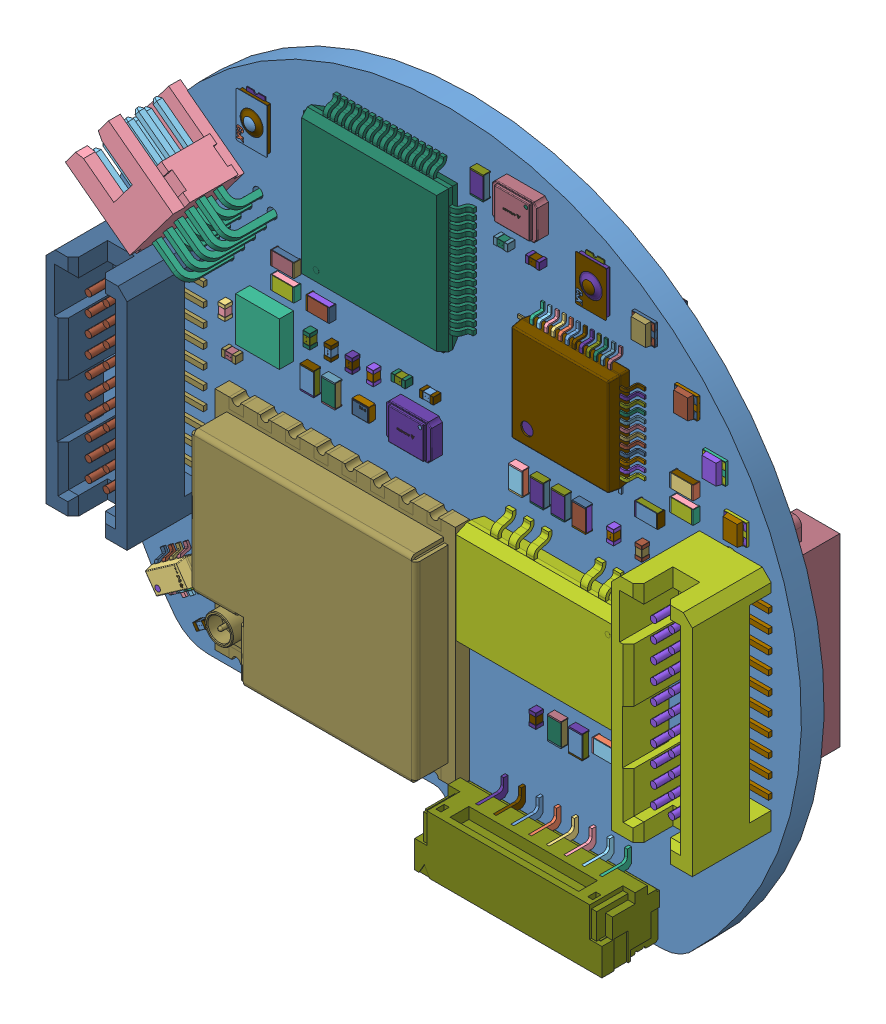
SolidWorks assembly HYDRA_V4_LINK_V2, configuration Default. Lengths in mm. (continued)
Components (placement in the parent): (continued)
- Open CASCADE STEP translator 7.5 367-1: Open CASCADE STEP translator 7.5 367 [Default] at origin size (0.95 1.45 0.05)
- Open CASCADE STEP translator 7.5 368-1: Open CASCADE STEP translator 7.5 368 [Default] at origin size (0.95 1.55 0.4)
- Open CASCADE STEP translator 7.5 369-1: Open CASCADE STEP translator 7.5 369 [Default] at origin size (0.95 0.1 0.5)
- Open CASCADE STEP translator 7.5 370-1: Open CASCADE STEP translator 7.5 370 [Default] at origin size (0.95 0.1 0.5)
- Open CASCADE STEP translator 7.5 371-1: Open CASCADE STEP translator 7.5 371 [Default] at origin size (0.95 1.45 0.05)
- Open CASCADE STEP translator 7.5 372-1: Open CASCADE STEP translator 7.5 372 [Default] at origin size (0.95 1.55 0.4)
- Open CASCADE STEP translator 7.5 373-1: Open CASCADE STEP translator 7.5 373 [Default] at origin size (0.95 0.1 0.5)
- Open CASCADE STEP translator 7.5 374-1: Open CASCADE STEP translator 7.5 374 [Default] at origin size (0.95 0.1 0.5)
- Open CASCADE STEP translator 7.5 375-1: Open CASCADE STEP translator 7.5 375 [Default] at origin size (0.95 1.45 0.05)
- Open CASCADE STEP translator 7.5 376-1: Open CASCADE STEP translator 7.5 376 [Default] at origin size (0.95 1.55 0.4)
- Open CASCADE STEP translator 7.5 377-1: Open CASCADE STEP translator 7.5 377 [Default] at origin size (0.95 0.1 0.5)
- Open CASCADE STEP translator 7.5 378-1: Open CASCADE STEP translator 7.5 378 [Default] at origin size (0.95 0.1 0.5)
- Open CASCADE STEP translator 7.5 379-1: Open CASCADE STEP translator 7.5 379 [Default] at origin size (0.95 1.45 0.05)
- Open CASCADE STEP translator 7.5 380-1: Open CASCADE STEP translator 7.5 380 [Default] at origin size (0.95 1.55 0.4)
- Open CASCADE STEP translator 7.5 381-1: Open CASCADE STEP translator 7.5 381 [Default] at origin size (0.95 0.1 0.5)
- Open CASCADE STEP translator 7.5 382-1: Open CASCADE STEP translator 7.5 382 [Default] at origin size (0.95 0.1 0.5)
- Open CASCADE STEP translator 7.5 383-1: Open CASCADE STEP translator 7.5 383 [Default] at origin size (0.95 1.45 0.05)
- Open CASCADE STEP translator 7.5 384-1: Open CASCADE STEP translator 7.5 384 [Default] at origin size (0.95 1.55 0.4)
- Open CASCADE STEP translator 7.5 385-1: Open CASCADE STEP translator 7.5 385 [Default] at origin size (0.95 0.1 0.5)
- Open CASCADE STEP translator 7.5 386-1: Open CASCADE STEP translator 7.5 386 [Default] at origin size (0.95 0.1 0.5)
- Open CASCADE STEP translator 7.5 387-1: Open CASCADE STEP translator 7.5 387 [Default] at origin size (0.95 1.45 0.05)
- Open CASCADE STEP translator 7.5 388-1: Open CASCADE STEP translator 7.5 388 [Default] at origin size (0.95 1.55 0.4)
- Open CASCADE STEP translator 7.5 389-1: Open CASCADE STEP translator 7.5 389 [Default] at origin size (0.95 0.1 0.5)
- Open CASCADE STEP translator 7.5 390-1: Open CASCADE STEP translator 7.5 390 [Default] at origin size (0.95 0.1 0.5)
- Open CASCADE STEP translator 7.5 391-1: Open CASCADE STEP translator 7.5 391 [Default] at origin size (0.95 1.45 0.05)
- Open CASCADE STEP translator 7.5 392-1: Open CASCADE STEP translator 7.5 392 [Default] at origin size (0.95 1.55 0.4)
- Open CASCADE STEP translator 7.5 393-1: Open CASCADE STEP translator 7.5 393 [Default] at origin size (0.95 0.1 0.5)
- Open CASCADE STEP translator 7.5 394-1: Open CASCADE STEP translator 7.5 394 [Default] at origin size (0.95 0.1 0.5)
- Open CASCADE STEP translator 7.5 395-1: Open CASCADE STEP translator 7.5 395 [Default] at origin size (0.95 1.45 0.05)
- Open CASCADE STEP translator 7.5 396-1: Open CASCADE STEP translator 7.5 396 [Default] at origin size (0.95 1.55 0.4)
- Open CASCADE STEP translator 7.5 397-1: Open CASCADE STEP translator 7.5 397 [Default] at origin size (0.95 0.1 0.5)
- Open CASCADE STEP translator 7.5 398-1: Open CASCADE STEP translator 7.5 398 [Default] at origin size (0.95 0.1 0.5)
- Open CASCADE STEP translator 7.5 399-1: Open CASCADE STEP translator 7.5 399 [Default] at origin size (0.95 1.45 0.05)
- Open CASCADE STEP translator 7.5 400-1: Open CASCADE STEP translator 7.5 400 [Default] at origin size (0.95 1.55 0.4)
- Open CASCADE STEP translator 7.5 401-1: Open CASCADE STEP translator 7.5 401 [Default] at origin size (0.95 0.1 0.5)
- Open CASCADE STEP translator 7.5 402-1: Open CASCADE STEP translator 7.5 402 [Default] at origin size (0.95 0.1 0.5)
- Open CASCADE STEP translator 7.5 403-1: Open CASCADE STEP translator 7.5 403 [Default] at origin size (0.95 1.45 0.05)
- Open CASCADE STEP translator 7.5 404-1: Open CASCADE STEP translator 7.5 404 [Default] at origin size (0.95 1.55 0.4)
- Open CASCADE STEP translator 7.5 405-1: Open CASCADE STEP translator 7.5 405 [Default] at origin size (0.95 0.1 0.5)
- Open CASCADE STEP translator 7.5 406-1: Open CASCADE STEP translator 7.5 406 [Default] at origin size (0.95 0.1 0.5)
- Open CASCADE STEP translator 7.5 407-1: Open CASCADE STEP translator 7.5 407 [Default] at origin size (0.95 1.45 0.05)
- Open CASCADE STEP translator 7.5 408-1: Open CASCADE STEP translator 7.5 408 [Default] at origin size (0.95 1.55 0.4)
- Open CASCADE STEP translator 7.5 409-1: Open CASCADE STEP translator 7.5 409 [Default] at origin size (0.95 0.1 0.5)
- Open CASCADE STEP translator 7.5 410-1: Open CASCADE STEP translator 7.5 410 [Default] at origin size (0.95 0.1 0.5)
- Open CASCADE STEP translator 7.5 411-1: Open CASCADE STEP translator 7.5 411 [Default] at origin size (0.95 1.45 0.05)
- Open CASCADE STEP translator 7.5 412-1: Open CASCADE STEP translator 7.5 412 [Default] at origin size (1.55 0.95 0.4)
- Open CASCADE STEP translator 7.5 413-1: Open CASCADE STEP translator 7.5 413 [Default] at origin size (0.1 0.95 0.5)
- Open CASCADE STEP translator 7.5 414-1: Open CASCADE STEP translator 7.5 414 [Default] at origin size (0.1 0.95 0.5)
- Open CASCADE STEP translator 7.5 415-1: Open CASCADE STEP translator 7.5 415 [Default] at origin size (1.45 0.95 0.05)
- Open CASCADE STEP translator 7.5 416-1: Open CASCADE STEP translator 7.5 416 [Default] at origin size (1.55 0.95 0.4)
- Open CASCADE STEP translator 7.5 417-1: Open CASCADE STEP translator 7.5 417 [Default] at origin size (0.1 0.95 0.5)
- Open CASCADE STEP translator 7.5 418-1: Open CASCADE STEP translator 7.5 418 [Default] at origin size (0.1 0.95 0.5)
- Open CASCADE STEP translator 7.5 419-1: Open CASCADE STEP translator 7.5 419 [Default] at origin size (1.45 0.95 0.05)
- Open CASCADE STEP translator 7.5 420-1: Open CASCADE STEP translator 7.5 420 [Default] at origin size (1.55 0.95 0.4)
- Open CASCADE STEP translator 7.5 421-1: Open CASCADE STEP translator 7.5 421 [Default] at origin size (0.1 0.95 0.5)
- Open CASCADE STEP translator 7.5 422-1: Open CASCADE STEP translator 7.5 422 [Default] at origin size (0.1 0.95 0.5)
- Open CASCADE STEP translator 7.5 423-1: Open CASCADE STEP translator 7.5 423 [Default] at origin size (1.45 0.95 0.05)
- Open CASCADE STEP translator 7.5 424-1: Open CASCADE STEP translator 7.5 424 [Default] at origin size (1.55 0.95 0.4)
- Open CASCADE STEP translator 7.5 425-1: Open CASCADE STEP translator 7.5 425 [Default] at origin size (0.1 0.95 0.5)
- Open CASCADE STEP translator 7.5 426-1: Open CASCADE STEP translator 7.5 426 [Default] at origin size (0.1 0.95 0.5)
- Open CASCADE STEP translator 7.5 427-1: Open CASCADE STEP translator 7.5 427 [Default] at origin size (1.45 0.95 0.05)
- Open CASCADE STEP translator 7.5 428-1: Open CASCADE STEP translator 7.5 428 [Default] at origin size (1.55 0.95 0.4)
- Open CASCADE STEP translator 7.5 429-1: Open CASCADE STEP translator 7.5 429 [Default] at origin size (0.1 0.95 0.5)
- Open CASCADE STEP translator 7.5 430-1: Open CASCADE STEP translator 7.5 430 [Default] at origin size (0.1 0.95 0.5)
- Open CASCADE STEP translator 7.5 431-1: Open CASCADE STEP translator 7.5 431 [Default] at origin size (1.45 0.95 0.05)
- Open CASCADE STEP translator 7.5 432-1: Open CASCADE STEP translator 7.5 432 [Default] at origin size (1.55 0.95 0.4)
- Open CASCADE STEP translator 7.5 433-1: Open CASCADE STEP translator 7.5 433 [Default] at origin size (0.1 0.95 0.5)
- Open CASCADE STEP translator 7.5 434-1: Open CASCADE STEP translator 7.5 434 [Default] at origin size (0.1 0.95 0.5)
- Open CASCADE STEP translator 7.5 435-1: Open CASCADE STEP translator 7.5 435 [Default] at origin size (1.45 0.95 0.05)
- Open CASCADE STEP translator 7.5 436-1: Open CASCADE STEP translator 7.5 436 [Default] at origin size (1.55 0.95 0.4)
- Open CASCADE STEP translator 7.5 437-1: Open CASCADE STEP translator 7.5 437 [Default] at origin size (0.1 0.95 0.5)
- Open CASCADE STEP translator 7.5 438-1: Open CASCADE STEP translator 7.5 438 [Default] at origin size (0.1 0.95 0.5)
- Open CASCADE STEP translator 7.5 439-1: Open CASCADE STEP translator 7.5 439 [Default] at origin size (1.45 0.95 0.05)
- Open CASCADE STEP translator 7.5 440-1: Open CASCADE STEP translator 7.5 440 [Default] at origin size (1.55 0.95 0.4)
- Open CASCADE STEP translator 7.5 441-1: Open CASCADE STEP translator 7.5 441 [Default] at origin size (0.1 0.95 0.5)
- Open CASCADE STEP translator 7.5 442-1: Open CASCADE STEP translator 7.5 442 [Default] at origin size (0.1 0.95 0.5)
- Open CASCADE STEP translator 7.5 443-1: Open CASCADE STEP translator 7.5 443 [Default] at origin size (1.45 0.95 0.05)
- Open CASCADE STEP translator 7.5 444-1: Open CASCADE STEP translator 7.5 444 [Default] at origin size (1.55 0.95 0.4)
- Open CASCADE STEP translator 7.5 445-1: Open CASCADE STEP translator 7.5 445 [Default] at origin size (0.1 0.95 0.5)
- Open CASCADE STEP translator 7.5 446-1: Open CASCADE STEP translator 7.5 446 [Default] at origin size (0.1 0.95 0.5)
- Open CASCADE STEP translator 7.5 447-1: Open CASCADE STEP translator 7.5 447 [Default] at origin size (1.45 0.95 0.05)
- Open CASCADE STEP translator 7.5 448-1: Open CASCADE STEP translator 7.5 448 [Default] at origin size (1.55 0.95 0.4)
- Open CASCADE STEP translator 7.5 449-1: Open CASCADE STEP translator 7.5 449 [Default] at origin size (0.1 0.95 0.5)
- Open CASCADE STEP translator 7.5 450-1: Open CASCADE STEP translator 7.5 450 [Default] at origin size (0.1 0.95 0.5)
- Open CASCADE STEP translator 7.5 451-1: Open CASCADE STEP translator 7.5 451 [Default] at origin size (1.45 0.95 0.05)
- Open CASCADE STEP translator 7.5 452-1: Open CASCADE STEP translator 7.5 452 [Default] at origin size (1.55 0.95 0.4)
- Open CASCADE STEP translator 7.5 453-1: Open CASCADE STEP translator 7.5 453 [Default] at origin size (0.1 0.95 0.5)
- Open CASCADE STEP translator 7.5 454-1: Open CASCADE STEP translator 7.5 454 [Default] at origin size (0.1 0.95 0.5)
- Open CASCADE STEP translator 7.5 455-1: Open CASCADE STEP translator 7.5 455 [Default] at origin size (1.45 0.95 0.05)
- Open CASCADE STEP translator 7.5 456-1: Open CASCADE STEP translator 7.5 456 [Default] at origin size (1.55 0.95 0.4)
- Open CASCADE STEP translator 7.5 457-1: Open CASCADE STEP translator 7.5 457 [Default] at origin size (0.1 0.95 0.5)
- Open CASCADE STEP translator 7.5 458-1: Open CASCADE STEP translator 7.5 458 [Default] at origin size (0.1 0.95 0.5)
- Open CASCADE STEP translator 7.5 459-1: Open CASCADE STEP translator 7.5 459 [Default] at origin size (1.45 0.95 0.05)
- Open CASCADE STEP translator 7.5 460-1: Open CASCADE STEP translator 7.5 460 [Default] at origin size (1.55 0.95 0.4)
- Open CASCADE STEP translator 7.5 461-1: Open CASCADE STEP translator 7.5 461 [Default] at origin size (0.1 0.95 0.5)
- Open CASCADE STEP translator 7.5 462-1: Open CASCADE STEP translator 7.5 462 [Default] at origin size (0.1 0.95 0.5)
- Open CASCADE STEP translator 7.5 463-1: Open CASCADE STEP translator 7.5 463 [Default] at origin size (1.45 0.95 0.05)
- Open CASCADE STEP translator 7.5 464-1: Open CASCADE STEP translator 7.5 464 [Default] at origin size (1.55 0.95 0.4)
- Open CASCADE STEP translator 7.5 465-1: Open CASCADE STEP translator 7.5 465 [Default] at origin size (0.1 0.95 0.5)
- Open CASCADE STEP translator 7.5 466-1: Open CASCADE STEP translator 7.5 466 [Default] at origin size (0.1 0.95 0.5)
- Open CASCADE STEP translator 7.5 467-1: Open CASCADE STEP translator 7.5 467 [Default] at origin size (1.45 0.95 0.05)
- Open CASCADE STEP translator 7.5 468-1: Open CASCADE STEP translator 7.5 468 [Default] at origin size (0.95 1.55 0.4)
- Open CASCADE STEP translator 7.5 469-1: Open CASCADE STEP translator 7.5 469 [Default] at origin size (0.95 0.1 0.5)
- Open CASCADE STEP translator 7.5 470-1: Open CASCADE STEP translator 7.5 470 [Default] at origin size (0.95 0.1 0.5)
- Open CASCADE STEP translator 7.5 471-1: Open CASCADE STEP translator 7.5 471 [Default] at origin size (0.95 1.45 0.05)
- Open CASCADE STEP translator 7.5 472-1: Open CASCADE STEP translator 7.5 472 [Default] at origin size (1.55 0.95 0.4)
- Open CASCADE STEP translator 7.5 473-1: Open CASCADE STEP translator 7.5 473 [Default] at origin size (0.1 0.95 0.5)
- Open CASCADE STEP translator 7.5 474-1: Open CASCADE STEP translator 7.5 474 [Default] at origin size (0.1 0.95 0.5)
- Open CASCADE STEP translator 7.5 475-1: Open CASCADE STEP translator 7.5 475 [Default] at origin size (1.45 0.95 0.05)
- Open CASCADE STEP translator 7.5 476-1: Open CASCADE STEP translator 7.5 476 [Default] at origin size (1.55 0.95 0.4)
- Open CASCADE STEP translator 7.5 477-1: Open CASCADE STEP translator 7.5 477 [Default] at origin size (0.1 0.95 0.5)
- Open CASCADE STEP translator 7.5 478-1: Open CASCADE STEP translator 7.5 478 [Default] at origin size (0.1 0.95 0.5)
- Open CASCADE STEP translator 7.5 479-1: Open CASCADE STEP translator 7.5 479 [Default] at origin size (1.45 0.95 0.05)
- Open CASCADE STEP translator 7.5 480-1: Open CASCADE STEP translator 7.5 480 [Default] at origin size (0.95 1.55 0.4)
- Open CASCADE STEP translator 7.5 481-1: Open CASCADE STEP translator 7.5 481 [Default] at origin size (0.95 0.1 0.5)
- Open CASCADE STEP translator 7.5 482-1: Open CASCADE STEP translator 7.5 482 [Default] at origin size (0.95 0.1 0.5)
- Open CASCADE STEP translator 7.5 483-1: Open CASCADE STEP translator 7.5 483 [Default] at origin size (0.95 1.45 0.05)
- Open CASCADE STEP translator 7.5 484-1: Open CASCADE STEP translator 7.5 484 [Default] at origin size (0.95 1.55 0.4)
- Open CASCADE STEP translator 7.5 485-1: Open CASCADE STEP translator 7.5 485 [Default] at origin size (0.95 0.1 0.5)
- Open CASCADE STEP translator 7.5 486-1: Open CASCADE STEP translator 7.5 486 [Default] at origin size (0.95 0.1 0.5)
- Open CASCADE STEP translator 7.5 487-1: Open CASCADE STEP translator 7.5 487 [Default] at origin size (0.95 1.45 0.05)
- Open CASCADE STEP translator 7.5 488-1: Open CASCADE STEP translator 7.5 488 [Default] at origin size (1.36 2.21 1.09)
- Open CASCADE STEP translator 7.5 489-1: Open CASCADE STEP translator 7.5 489 [Default] at origin size (0.43 0.4 0.59)
- Open CASCADE STEP translator 7.5 490-1: Open CASCADE STEP translator 7.5 490 [Default] at origin size (0.43 0.4 0.59)
- Open CASCADE STEP translator 7.5 491-1: Open CASCADE STEP translator 7.5 491 [Default] at origin size (0.43 0.4 0.59)
- Open CASCADE STEP translator 7.5 492-1: Open CASCADE STEP translator 7.5 492 [Default] at origin size (1.25 2 0.96)
- Open CASCADE STEP translator 7.5 493-1: Open CASCADE STEP translator 7.5 493 [Default] at origin size (0.8 0.2 0.75)
- Open CASCADE STEP translator 7.5 494-1: Open CASCADE STEP translator 7.5 494 [Default] at origin size (0.8 0.2 0.75)
- Open CASCADE STEP translator 7.5 495-1: Open CASCADE STEP translator 7.5 495 [Default] at origin size (0.8 0.2 0.75)
- Open CASCADE STEP translator 7.5 496-1: Open CASCADE STEP translator 7.5 496 [Default] at origin size (0.25 0.25 0.01)
- Open CASCADE STEP translator 7.5 497-1: Open CASCADE STEP translator 7.5 497 [Default] at origin size (0.8 0.2 0.75)
- Open CASCADE STEP translator 7.5 498-1: Open CASCADE STEP translator 7.5 498 [Default] at origin size (0.8 0.2 0.75)
- Open CASCADE STEP translator 7.5 499-1: Open CASCADE STEP translator 7.5 499 [Default] at origin size (0.8 0.2 0.75)
- Open CASCADE STEP translator 7.5 500-1: Open CASCADE STEP translator 7.5 500 [Default] at origin size (0.96 0.16 0.01)
- Open CASCADE STEP translator 7.5 501-1: Open CASCADE STEP translator 7.5 501 [Default] at origin size (1.36 2.21 1.09)
- Open CASCADE STEP translator 7.5 502-1: Open CASCADE STEP translator 7.5 502 [Default] at origin size (0.43 0.4 0.59)
- Open CASCADE STEP translator 7.5 503-1: Open CASCADE STEP translator 7.5 503 [Default] at origin size (0.43 0.4 0.59)
- Open CASCADE STEP translator 7.5 504-1: Open CASCADE STEP translator 7.5 504 [Default] at origin size (0.43 0.4 0.59)
- Open CASCADE STEP translator 7.5 505-1: Open CASCADE STEP translator 7.5 505 [Default] at origin size (2.21 1.36 1.09)
- Open CASCADE STEP translator 7.5 506-1: Open CASCADE STEP translator 7.5 506 [Default] at origin size (0.4 0.43 0.59)
- Open CASCADE STEP translator 7.5 507-1: Open CASCADE STEP translator 7.5 507 [Default] at origin size (0.4 0.43 0.59)
- Open CASCADE STEP translator 7.5 508-1: Open CASCADE STEP translator 7.5 508 [Default] at origin size (0.4 0.43 0.59)
- Open CASCADE STEP translator 7.5 509-1: Open CASCADE STEP translator 7.5 509 [Default] at origin size (4.07 4.06 1.2)
- Open CASCADE STEP translator 7.5 510-1: Open CASCADE STEP translator 7.5 510 [Default] at origin size (2 4.45 0.9)
- Open CASCADE STEP translator 7.5 511-1: Open CASCADE STEP translator 7.5 511 [Default] at origin size (1.26 1.48 0.01)
- Open CASCADE STEP translator 7.5 512-1: Open CASCADE STEP translator 7.5 512 [Default] at origin size (3.99 3.99 0.1)
- Open CASCADE STEP translator 7.5 513-1: Open CASCADE STEP translator 7.5 513 [Default] at origin size (4.06 4.07 1.2)
- Open CASCADE STEP translator 7.5 514-1: Open CASCADE STEP translator 7.5 514 [Default] at origin size (4.45 2 0.9)
- Open CASCADE STEP translator 7.5 515-1: Open CASCADE STEP translator 7.5 515 [Default] at origin size (1.48 1.26 0.01)
- Open CASCADE STEP translator 7.5 516-1: Open CASCADE STEP translator 7.5 516 [Default] at origin size (3.99 3.99 0.1)
- Open CASCADE STEP translator 7.5 517-1: Open CASCADE STEP translator 7.5 517 [Default] at origin size (0.5 1 0.55)
- Open CASCADE STEP translator 7.5 518-1: Open CASCADE STEP translator 7.5 518 [Default] at origin size (0.49 0.5 0.54)
- Open CASCADE STEP translator 7.5 519-1: Open CASCADE STEP translator 7.5 519 [Default] at origin size (0.06 0.26 0.01)
- Open CASCADE STEP translator 7.5 520-1: Open CASCADE STEP translator 7.5 520 [Default] at origin size (0.5 1 0.55)
- Open CASCADE STEP translator 7.5 521-1: Open CASCADE STEP translator 7.5 521 [Default] at origin size (0.49 0.5 0.54)
- Open CASCADE STEP translator 7.5 522-1: Open CASCADE STEP translator 7.5 522 [Default] at origin size (0.06 0.26 0.01)
- Open CASCADE STEP translator 7.5 523-1: Open CASCADE STEP translator 7.5 523 [Default] at origin size (2.15 1.35 0.85)
- Open CASCADE STEP translator 7.5 524-1: Open CASCADE STEP translator 7.5 524 [Default] at origin size (2.15 1.35 0.85)
- Open CASCADE STEP translator 7.5 525-1: Open CASCADE STEP translator 7.5 525 [Default] at origin size (1.21 0.73 0.02)
- Open CASCADE STEP translator 7.5 526-1: Open CASCADE STEP translator 7.5 526 [Default] at origin size (1.35 2.15 0.85)
- Open CASCADE STEP translator 7.5 527-1: Open CASCADE STEP translator 7.5 527 [Default] at origin size (1.35 2.15 0.85)
- Open CASCADE STEP translator 7.5 528-1: Open CASCADE STEP translator 7.5 528 [Default] at origin size (0.73 1.21 0.02)
- Open CASCADE STEP translator 7.5 529-1: Open CASCADE STEP translator 7.5 529 [Default] at origin size (1.6 1.5 0.2)
- Open CASCADE STEP translator 7.5 530-1: Open CASCADE STEP translator 7.5 530 [Default] at origin size (1.6 1.4 0.19)
- Open CASCADE STEP translator 7.5 531-1: Open CASCADE STEP translator 7.5 531 [Default] at origin size (1.1 1.5 0.36)
- Open CASCADE STEP translator 7.5 532-1: Open CASCADE STEP translator 7.5 532 [Default] at origin size (1.6 1.5 0.2)
- Open CASCADE STEP translator 7.5 533-1: Open CASCADE STEP translator 7.5 533 [Default] at origin size (1.6 1.4 0.19)
- Open CASCADE STEP translator 7.5 534-1: Open CASCADE STEP translator 7.5 534 [Default] at origin size (1.1 1.5 0.36)
- Open CASCADE STEP translator 7.5 535-1: Open CASCADE STEP translator 7.5 535 [Default] at origin size (0.8 1.2 0.7)
- Open CASCADE STEP translator 7.5 536-1: Open CASCADE STEP translator 7.5 536 [Default] at origin size (0.5 1 0.55)
- Open CASCADE STEP translator 7.5 537-1: Open CASCADE STEP translator 7.5 537 [Default] at origin size (0.47 0.5 0.52)
- Open CASCADE STEP translator 7.5 538-1: Open CASCADE STEP translator 7.5 538 [Default] at origin size (0.03 0.3 0)
- Open CASCADE STEP translator 7.5 539-1: Open CASCADE STEP translator 7.5 539 [Default] at origin size (0.5 1 0.55)
- Open CASCADE STEP translator 7.5 540-1: Open CASCADE STEP translator 7.5 540 [Default] at origin size (0.47 0.5 0.52)
- Open CASCADE STEP translator 7.5 541-1: Open CASCADE STEP translator 7.5 541 [Default] at origin size (0.03 0.3 0)
- Open CASCADE STEP translator 7.5 542-1: Open CASCADE STEP translator 7.5 542 [Default] at origin size (0.5 1 0.55)
- Open CASCADE STEP translator 7.5 543-1: Open CASCADE STEP translator 7.5 543 [Default] at origin size (0.47 0.5 0.52)
- Open CASCADE STEP translator 7.5 544-1: Open CASCADE STEP translator 7.5 544 [Default] at origin size (0.03 0.3 0)
- Open CASCADE STEP translator 7.5 545-1: Open CASCADE STEP translator 7.5 545 [Default] at origin size (0.5 1 0.55)
- Open CASCADE STEP translator 7.5 546-1: Open CASCADE STEP translator 7.5 546 [Default] at origin size (0.47 0.5 0.52)
- Open CASCADE STEP translator 7.5 547-1: Open CASCADE STEP translator 7.5 547 [Default] at origin size (0.03 0.3 0)
- Open CASCADE STEP translator 7.5 548-1: Open CASCADE STEP translator 7.5 548 [Default] at origin size (0.5 1 0.55)
- Open CASCADE STEP translator 7.5 549-1: Open CASCADE STEP translator 7.5 549 [Default] at origin size (0.47 0.5 0.52)
- Open CASCADE STEP translator 7.5 550-1: Open CASCADE STEP translator 7.5 550 [Default] at origin size (0.03 0.3 0)
- Open CASCADE STEP translator 7.5 551-1: Open CASCADE STEP translator 7.5 551 [Default] at origin size (0.5 1 0.55)
- Open CASCADE STEP translator 7.5 552-1: Open CASCADE STEP translator 7.5 552 [Default] at origin size (0.47 0.5 0.52)
- Open CASCADE STEP translator 7.5 553-1: Open CASCADE STEP translator 7.5 553 [Default] at origin size (0.03 0.3 0)
- Open CASCADE STEP translator 7.5 554-1: Open CASCADE STEP translator 7.5 554 [Default] at origin size (0.5 1 0.55)
- Open CASCADE STEP translator 7.5 555-1: Open CASCADE STEP translator 7.5 555 [Default] at origin size (0.47 0.5 0.52)
- Open CASCADE STEP translator 7.5 556-1: Open CASCADE STEP translator 7.5 556 [Default] at origin size (0.03 0.3 0)
- Open CASCADE STEP translator 7.5 557-1: Open CASCADE STEP translator 7.5 557 [Default] at origin size (0.5 1 0.55)
- Open CASCADE STEP translator 7.5 558-1: Open CASCADE STEP translator 7.5 558 [Default] at origin size (0.47 0.5 0.52)
- Open CASCADE STEP translator 7.5 559-1: Open CASCADE STEP translator 7.5 559 [Default] at origin size (0.03 0.3 0)
- Open CASCADE STEP translator 7.5 560-1: Open CASCADE STEP translator 7.5 560 [Default] at origin size (0.5 1 0.55)
- Open CASCADE STEP translator 7.5 561-1: Open CASCADE STEP translator 7.5 561 [Default] at origin size (0.47 0.5 0.52)
- Open CASCADE STEP translator 7.5 562-1: Open CASCADE STEP translator 7.5 562 [Default] at origin size (0.03 0.3 0)
- Open CASCADE STEP translator 7.5 563-1: Open CASCADE STEP translator 7.5 563 [Default] at origin size (0.5 1 0.55)
- Open CASCADE STEP translator 7.5 564-1: Open CASCADE STEP translator 7.5 564 [Default] at origin size (0.47 0.5 0.52)
- Open CASCADE STEP translator 7.5 565-1: Open CASCADE STEP translator 7.5 565 [Default] at origin size (0.03 0.3 0)
- Open CASCADE STEP translator 7.5 566-1: Open CASCADE STEP translator 7.5 566 [Default] at origin size (0.5 1 0.55)
- Open CASCADE STEP translator 7.5 567-1: Open CASCADE STEP translator 7.5 567 [Default] at origin size (0.47 0.5 0.52)
- Open CASCADE STEP translator 7.5 568-1: Open CASCADE STEP translator 7.5 568 [Default] at origin size (0.03 0.3 0)
- Open CASCADE STEP translator 7.5 569-1: Open CASCADE STEP translator 7.5 569 [Default] at origin size (0.5 1 0.55)
- Open CASCADE STEP translator 7.5 570-1: Open CASCADE STEP translator 7.5 570 [Default] at origin size (0.47 0.5 0.52)
- Open CASCADE STEP translator 7.5 571-1: Open CASCADE STEP translator 7.5 571 [Default] at origin size (0.03 0.3 0)
- Open CASCADE STEP translator 7.5 572-1: Open CASCADE STEP translator 7.5 572 [Default] at origin size (1 0.5 0.55)
- Open CASCADE STEP translator 7.5 573-1: Open CASCADE STEP translator 7.5 573 [Default] at origin size (0.5 0.47 0.52)
- Open CASCADE STEP translator 7.5 574-1: Open CASCADE STEP translator 7.5 574 [Default] at origin size (0.3 0.03 0)
- Open CASCADE STEP translator 7.5 575-1: Open CASCADE STEP translator 7.5 575 [Default] at origin size (1 0.5 0.55)
- Open CASCADE STEP translator 7.5 576-1: Open CASCADE STEP translator 7.5 576 [Default] at origin size (0.5 0.47 0.52)
- Open CASCADE STEP translator 7.5 577-1: Open CASCADE STEP translator 7.5 577 [Default] at origin size (0.3 0.03 0)
- Open CASCADE STEP translator 7.5 578-1: Open CASCADE STEP translator 7.5 578 [Default] at origin size (1 0.5 0.55)
- Open CASCADE STEP translator 7.5 579-1: Open CASCADE STEP translator 7.5 579 [Default] at origin size (0.5 0.47 0.52)
- Open CASCADE STEP translator 7.5 580-1: Open CASCADE STEP translator 7.5 580 [Default] at origin size (0.3 0.03 0)
- Open CASCADE STEP translator 7.5 581-1: Open CASCADE STEP translator 7.5 581 [Default] at origin size (1 0.5 0.55)
- Open CASCADE STEP translator 7.5 582-1: Open CASCADE STEP translator 7.5 582 [Default] at origin size (0.5 0.47 0.52)
- Open CASCADE STEP translator 7.5 583-1: Open CASCADE STEP translator 7.5 583 [Default] at origin size (0.3 0.03 0)
- Open CASCADE STEP translator 7.5 584-1: Open CASCADE STEP translator 7.5 584 [Default] at origin size (0.5 1 0.55)
- Open CASCADE STEP translator 7.5 585-1: Open CASCADE STEP translator 7.5 585 [Default] at origin size (0.47 0.5 0.52)
- Open CASCADE STEP translator 7.5 586-1: Open CASCADE STEP translator 7.5 586 [Default] at origin size (0.03 0.3 0)
- Open CASCADE STEP translator 7.5 587-1: Open CASCADE STEP translator 7.5 587 [Default] at origin size (0.5 1 0.55)
- Open CASCADE STEP translator 7.5 588-1: Open CASCADE STEP translator 7.5 588 [Default] at origin size (0.47 0.5 0.52)
- Open CASCADE STEP translator 7.5 589-1: Open CASCADE STEP translator 7.5 589 [Default] at origin size (0.03 0.3 0)
- Open CASCADE STEP translator 7.5 590-1: Open CASCADE STEP translator 7.5 590 [Default] at origin size (1 0.5 0.55)
- Open CASCADE STEP translator 7.5 591-1: Open CASCADE STEP translator 7.5 591 [Default] at origin size (0.5 0.47 0.52)
- Open CASCADE STEP translator 7.5 592-1: Open CASCADE STEP translator 7.5 592 [Default] at origin size (0.3 0.03 0)
- Open CASCADE STEP translator 7.5 593-1: Open CASCADE STEP translator 7.5 593 [Default] at origin size (1 0.5 0.55)
- Open CASCADE STEP translator 7.5 594-1: Open CASCADE STEP translator 7.5 594 [Default] at origin size (0.5 0.47 0.52)
- Open CASCADE STEP translator 7.5 595-1: Open CASCADE STEP translator 7.5 595 [Default] at origin size (0.3 0.03 0)
- Open CASCADE STEP translator 7.5 596-1: Open CASCADE STEP translator 7.5 596 [Default] at origin size (1 0.5 0.55)
- Open CASCADE STEP translator 7.5 597-1: Open CASCADE STEP translator 7.5 597 [Default] at origin size (0.5 0.47 0.52)
- Open CASCADE STEP translator 7.5 598-1: Open CASCADE STEP translator 7.5 598 [Default] at origin size (0.3 0.03 0)
- Open CASCADE STEP translator 7.5 599-1: Open CASCADE STEP translator 7.5 599 [Default] at origin size (0.5 1 0.55)
- Open CASCADE STEP translator 7.5 600-1: Open CASCADE STEP translator 7.5 600 [Default] at origin size (0.47 0.5 0.52)
- Open CASCADE STEP translator 7.5 601-1: Open CASCADE STEP translator 7.5 601 [Default] at origin size (0.03 0.3 0)
- Open CASCADE STEP translator 7.5 602-1: Open CASCADE STEP translator 7.5 602 [Default] at origin size (0.5 1 0.55)
- Open CASCADE STEP translator 7.5 603-1: Open CASCADE STEP translator 7.5 603 [Default] at origin size (0.47 0.5 0.52)
- Open CASCADE STEP translator 7.5 604-1: Open CASCADE STEP translator 7.5 604 [Default] at origin size (0.03 0.3 0)
- Open CASCADE STEP translator 7.5 605-1: Open CASCADE STEP translator 7.5 605 [Default] at origin size (0.5 1 0.55)
- Open CASCADE STEP translator 7.5 606-1: Open CASCADE STEP translator 7.5 606 [Default] at origin size (0.47 0.5 0.52)
- Open CASCADE STEP translator 7.5 607-1: Open CASCADE STEP translator 7.5 607 [Default] at origin size (0.03 0.3 0)
- Open CASCADE STEP translator 7.5 608-1: Open CASCADE STEP translator 7.5 608 [Default] at origin size (1 0.5 0.55)
- Open CASCADE STEP translator 7.5 609-1: Open CASCADE STEP translator 7.5 609 [Default] at origin size (0.5 0.47 0.52)
- Open CASCADE STEP translator 7.5 610-1: Open CASCADE STEP translator 7.5 610 [Default] at origin size (0.3 0.03 0)
- Open CASCADE STEP translator 7.5 611-1: Open CASCADE STEP translator 7.5 611 [Default] at origin size (0.5 1 0.55)
- Open CASCADE STEP translator 7.5 612-1: Open CASCADE STEP translator 7.5 612 [Default] at origin size (0.47 0.5 0.52)
- Open CASCADE STEP translator 7.5 613-1: Open CASCADE STEP translator 7.5 613 [Default] at origin size (0.03 0.3 0)
- Open CASCADE STEP translator 7.5 614-1: Open CASCADE STEP translator 7.5 614 [Default] at origin size (0.5 1 0.55)
- Open CASCADE STEP translator 7.5 615-1: Open CASCADE STEP translator 7.5 615 [Default] at origin size (0.47 0.5 0.52)
- Open CASCADE STEP translator 7.5 616-1: Open CASCADE STEP translator 7.5 616 [Default] at origin size (0.03 0.3 0)
- Open CASCADE STEP translator 7.5 617-1: Open CASCADE STEP translator 7.5 617 [Default] at origin size (1 0.5 0.55)
- Open CASCADE STEP translator 7.5 618-1: Open CASCADE STEP translator 7.5 618 [Default] at origin size (0.5 0.47 0.52)
- Open CASCADE STEP translator 7.5 619-1: Open CASCADE STEP translator 7.5 619 [Default] at origin size (0.3 0.03 0)
- Open CASCADE STEP translator 7.5 620-1: Open CASCADE STEP translator 7.5 620 [Default] at origin size (0.5 1 0.55)
- Open CASCADE STEP translator 7.5 621-1: Open CASCADE STEP translator 7.5 621 [Default] at origin size (0.47 0.5 0.52)
- Open CASCADE STEP translator 7.5 622-1: Open CASCADE STEP translator 7.5 622 [Default] at origin size (0.03 0.3 0)
- Open CASCADE STEP translator 7.5 623-1: Open CASCADE STEP translator 7.5 623 [Default] at origin size (0.5 1 0.55)
- Open CASCADE STEP translator 7.5 624-1: Open CASCADE STEP translator 7.5 624 [Default] at origin size (0.47 0.5 0.52)
- Open CASCADE STEP translator 7.5 625-1: Open CASCADE STEP translator 7.5 625 [Default] at origin size (0.03 0.3 0)
- Open CASCADE STEP translator 7.5 626-1: Open CASCADE STEP translator 7.5 626 [Default] at origin size (2.8 3.3 2)
- Open CASCADE STEP translator 7.5 627-1: Open CASCADE STEP translator 7.5 627 [Default] at origin size (2.2 0.8 1)
- Open CASCADE STEP translator 7.5 628-1: Open CASCADE STEP translator 7.5 628 [Default] at origin size (2.2 0.8 1)
- Open CASCADE STEP translator 7.5 629-1: Open CASCADE STEP translator 7.5 629 [Default] at origin size (2.11 2.66 0.01)
- Open CASCADE STEP translator 7.5 630-1: Open CASCADE STEP translator 7.5 630 [Default] at origin size (1 0.5 0.55)
- Open CASCADE STEP translator 7.5 631-1: Open CASCADE STEP translator 7.5 631 [Default] at origin size (0.5 0.47 0.52)
- Open CASCADE STEP translator 7.5 632-1: Open CASCADE STEP translator 7.5 632 [Default] at origin size (0.3 0.03 0)
- Open CASCADE STEP translator 7.5 633-1: Open CASCADE STEP translator 7.5 633 [Default] at origin size (1 0.5 0.55)
- Open CASCADE STEP translator 7.5 634-1: Open CASCADE STEP translator 7.5 634 [Default] at origin size (0.5 0.47 0.52)
- Open CASCADE STEP translator 7.5 635-1: Open CASCADE STEP translator 7.5 635 [Default] at origin size (0.3 0.03 0)
- Open CASCADE STEP translator 7.5 636-1: Open CASCADE STEP translator 7.5 636 [Default] at origin size (2.01 1.26 1.46)
- Open CASCADE STEP translator 7.5 637-1: Open CASCADE STEP translator 7.5 637 [Default] at origin size (1 1.25 1.45)
- Open CASCADE STEP translator 7.5 638-1: Open CASCADE STEP translator 7.5 638 [Default] at origin size (0.67 0.05 0.01)
- Open CASCADE STEP translator 7.5 639-1: Open CASCADE STEP translator 7.5 639 [Default] at origin size (1.1 1.25 1.45)
- Open CASCADE STEP translator 7.5 640-1: Open CASCADE STEP translator 7.5 640 [Default] at origin size (0.46 1.26 1.46)
- Open CASCADE STEP translator 7.5 641-1: Open CASCADE STEP translator 7.5 641 [Default] at origin size (0.46 1.26 1.46)
- Open CASCADE STEP translator 7.5 642-1: Open CASCADE STEP translator 7.5 642 [Default] at origin size (0.61 0.15 0.01)
- Open CASCADE STEP translator 7.5 643-1: Open CASCADE STEP translator 7.5 643 [Default] at origin size (1.1 1.25 1.45)
- Open CASCADE STEP translator 7.5 644-1: Open CASCADE STEP translator 7.5 644 [Default] at origin size (0.46 1.26 1.46)
- Open CASCADE STEP translator 7.5 645-1: Open CASCADE STEP translator 7.5 645 [Default] at origin size (0.46 1.26 1.46)
- Open CASCADE STEP translator 7.5 646-1: Open CASCADE STEP translator 7.5 646 [Default] at origin size (0.61 0.15 0.01)
- Open CASCADE STEP translator 7.5 647-1: Open CASCADE STEP translator 7.5 647 [Default] at origin size (1 0.5 0.55)
- Open CASCADE STEP translator 7.5 648-1: Open CASCADE STEP translator 7.5 648 [Default] at origin size (0.5 0.47 0.52)
- Open CASCADE STEP translator 7.5 649-1: Open CASCADE STEP translator 7.5 649 [Default] at origin size (0.3 0.03 0)
- Open CASCADE STEP translator 7.5 650-1: Open CASCADE STEP translator 7.5 650 [Default] at origin size (0.5 1 0.55)
- Open CASCADE STEP translator 7.5 651-1: Open CASCADE STEP translator 7.5 651 [Default] at origin size (0.47 0.5 0.52)
- Open CASCADE STEP translator 7.5 652-1: Open CASCADE STEP translator 7.5 652 [Default] at origin size (0.03 0.3 0)
- Open CASCADE STEP translator 7.5 653-1: Open CASCADE STEP translator 7.5 653 [Default] at origin size (0.5 1 0.55)
- Open CASCADE STEP translator 7.5 654-1: Open CASCADE STEP translator 7.5 654 [Default] at origin size (0.47 0.5 0.52)
- Open CASCADE STEP translator 7.5 655-1: Open CASCADE STEP translator 7.5 655 [Default] at origin size (0.03 0.3 0)
- Open CASCADE STEP translator 7.5 656-1: Open CASCADE STEP translator 7.5 656 [Default] at origin size (0.5 1 0.55)
- Open CASCADE STEP translator 7.5 657-1: Open CASCADE STEP translator 7.5 657 [Default] at origin size (0.47 0.5 0.52)
- Open CASCADE STEP translator 7.5 658-1: Open CASCADE STEP translator 7.5 658 [Default] at origin size (0.03 0.3 0)
- Open CASCADE STEP translator 7.5 659-1: Open CASCADE STEP translator 7.5 659 [Default] at origin size (0.5 1 0.55)
- Open CASCADE STEP translator 7.5 660-1: Open CASCADE STEP translator 7.5 660 [Default] at origin size (0.47 0.5 0.52)
- Open CASCADE STEP translator 7.5 661-1: Open CASCADE STEP translator 7.5 661 [Default] at origin size (0.03 0.3 0)
- Open CASCADE STEP translator 7.5 662-1: Open CASCADE STEP translator 7.5 662 [Default] at origin size (3.3 2.8 2)
- Open CASCADE STEP translator 7.5 663-1: Open CASCADE STEP translator 7.5 663 [Default] at origin size (0.8 2.2 1)
- Open CASCADE STEP translator 7.5 664-1: Open CASCADE STEP translator 7.5 664 [Default] at origin size (0.8 2.2 1)
- Open CASCADE STEP translator 7.5 665-1: Open CASCADE STEP translator 7.5 665 [Default] at origin size (2.66 2.11 0.01)
- Open CASCADE STEP translator 7.5 666-1: Open CASCADE STEP translator 7.5 666 [Default] at origin size (0.5 1 0.55)
- Open CASCADE STEP translator 7.5 667-1: Open CASCADE STEP translator 7.5 667 [Default] at origin size (0.47 0.5 0.52)
- Open CASCADE STEP translator 7.5 668-1: Open CASCADE STEP translator 7.5 668 [Default] at origin size (0.03 0.3 0)
- Open CASCADE STEP translator 7.5 669-1: Open CASCADE STEP translator 7.5 669 [Default] at origin size (1.27 2.02 1.42)
- Open CASCADE STEP translator 7.5 670-1: Open CASCADE STEP translator 7.5 670 [Default] at origin size (1.25 2 1.4)
- Open CASCADE STEP translator 7.5 671-1: Open CASCADE STEP translator 7.5 671 [Default] at origin size (0.12 0.53 0.1)
- Open CASCADE STEP translator 7.5 672-1: Open CASCADE STEP translator 7.5 672 [Default] at origin size (1.27 2.02 1.42)
- Open CASCADE STEP translator 7.5 673-1: Open CASCADE STEP translator 7.5 673 [Default] at origin size (1.25 2 1.4)
- Open CASCADE STEP translator 7.5 674-1: Open CASCADE STEP translator 7.5 674 [Default] at origin size (0.12 0.53 0.1)
- Open CASCADE STEP translator 7.5 675-1: Open CASCADE STEP translator 7.5 675 [Default] at origin size (1.27 2.02 1.42)
- Open CASCADE STEP translator 7.5 676-1: Open CASCADE STEP translator 7.5 676 [Default] at origin size (1.25 2 1.4)
- Open CASCADE STEP translator 7.5 677-1: Open CASCADE STEP translator 7.5 677 [Default] at origin size (0.12 0.53 0.1)
- Open CASCADE STEP translator 7.5 678-1: Open CASCADE STEP translator 7.5 678 [Default] at origin size (1.25 0.5 1.4)
- Open CASCADE STEP translator 7.5 679-1: Open CASCADE STEP translator 7.5 679 [Default] at origin size (1.25 0.5 1.4)
- Open CASCADE STEP translator 7.5 680-1: Open CASCADE STEP translator 7.5 680 [Default] at origin size (1.15 1 1.3)
- Open CASCADE STEP translator 7.5 681-1: Open CASCADE STEP translator 7.5 681 [Default] at origin size (1.25 0.5 1.4)
- Open CASCADE STEP translator 7.5 682-1: Open CASCADE STEP translator 7.5 682 [Default] at origin size (1.25 0.5 1.4)
- Open CASCADE STEP translator 7.5 683-1: Open CASCADE STEP translator 7.5 683 [Default] at origin size (1.15 1 1.3)
- Open CASCADE STEP translator 7.5 684-1: Open CASCADE STEP translator 7.5 684 [Default] at origin size (0.5 1 0.55)
- Open CASCADE STEP translator 7.5 685-1: Open CASCADE STEP translator 7.5 685 [Default] at origin size (0.47 0.5 0.52)
- Open CASCADE STEP translator 7.5 686-1: Open CASCADE STEP translator 7.5 686 [Default] at origin size (0.03 0.3 0)
- Open CASCADE STEP translator 7.5 687-1: Open CASCADE STEP translator 7.5 687 [Default] at origin size (0.5 1.25 1.4)
- Open CASCADE STEP translator 7.5 688-1: Open CASCADE STEP translator 7.5 688 [Default] at origin size (0.5 1.25 1.4)
- Open CASCADE STEP translator 7.5 689-1: Open CASCADE STEP translator 7.5 689 [Default] at origin size (1 1.15 1.3)
- Open CASCADE STEP translator 7.5 690-1: Open CASCADE STEP translator 7.5 690 [Default] at origin size (0.5 1 0.55)
- Open CASCADE STEP translator 7.5 691-1: Open CASCADE STEP translator 7.5 691 [Default] at origin size (0.47 0.5 0.52)
- Open CASCADE STEP translator 7.5 692-1: Open CASCADE STEP translator 7.5 692 [Default] at origin size (0.03 0.3 0)
- Open CASCADE STEP translator 7.5 693-1: Open CASCADE STEP translator 7.5 693 [Default] at origin size (1 0.5 0.55)
- Open CASCADE STEP translator 7.5 694-1: Open CASCADE STEP translator 7.5 694 [Default] at origin size (0.5 0.47 0.52)
- Open CASCADE STEP translator 7.5 695-1: Open CASCADE STEP translator 7.5 695 [Default] at origin size (0.3 0.03 0)
- Open CASCADE STEP translator 7.5 696-1: Open CASCADE STEP translator 7.5 696 [Default] at origin size (1 0.5 0.55)
- Open CASCADE STEP translator 7.5 697-1: Open CASCADE STEP translator 7.5 697 [Default] at origin size (0.5 0.47 0.52)
- Open CASCADE STEP translator 7.5 698-1: Open CASCADE STEP translator 7.5 698 [Default] at origin size (0.3 0.03 0)
- Open CASCADE STEP translator 7.5 699-1: Open CASCADE STEP translator 7.5 699 [Default] at origin size (0.5 1 0.55)
- Open CASCADE STEP translator 7.5 700-1: Open CASCADE STEP translator 7.5 700 [Default] at origin size (0.47 0.5 0.52)
- Open CASCADE STEP translator 7.5 701-1: Open CASCADE STEP translator 7.5 701 [Default] at origin size (0.03 0.3 0)
- Open CASCADE STEP translator 7.5 702-1: Open CASCADE STEP translator 7.5 702 [Default] at origin size (0.5 1 0.55)
- Open CASCADE STEP translator 7.5 703-1: Open CASCADE STEP translator 7.5 703 [Default] at origin size (0.47 0.5 0.52)
- Open CASCADE STEP translator 7.5 704-1: Open CASCADE STEP translator 7.5 704 [Default] at origin size (0.03 0.3 0)
- Open CASCADE STEP translator 7.5 705-1: Open CASCADE STEP translator 7.5 705 [Default] at origin size (0.5 1 0.55)
- Open CASCADE STEP translator 7.5 706-1: Open CASCADE STEP translator 7.5 706 [Default] at origin size (0.47 0.5 0.52)
- Open CASCADE STEP translator 7.5 707-1: Open CASCADE STEP translator 7.5 707 [Default] at origin size (0.03 0.3 0)
- Open CASCADE STEP translator 7.5 708-1: Open CASCADE STEP translator 7.5 708 [Default] at origin size (1.6 1.5 0.2)
- Open CASCADE STEP translator 7.5 709-1: Open CASCADE STEP translator 7.5 709 [Default] at origin size (1.6 1.4 0.19)
- Open CASCADE STEP translator 7.5 710-1: Open CASCADE STEP translator 7.5 710 [Default] at origin size (1.1 1.5 0.36)
- Open CASCADE STEP translator 7.5 711-1: Open CASCADE STEP translator 7.5 711 [Default] at origin size (1.6 1.5 0.2)
- Open CASCADE STEP translator 7.5 712-1: Open CASCADE STEP translator 7.5 712 [Default] at origin size (1.6 1.4 0.19)
- Open CASCADE STEP translator 7.5 713-1: Open CASCADE STEP translator 7.5 713 [Default] at origin size (1.1 1.5 0.36)
- Open CASCADE STEP translator 7.5 714-1: Open CASCADE STEP translator 7.5 714 [Default] at origin size (17 16 3.32)
- Open CASCADE STEP translator 7.5 715-1: Open CASCADE STEP translator 7.5 715 [Default] at origin size (3.68 15.88 5.84)
- Open CASCADE STEP translator 7.5 716-1: Open CASCADE STEP translator 7.5 716 [Default] at origin size (4.09 12.7 1.18)
- Open CASCADE STEP translator 7.5 717-1: Open CASCADE STEP translator 7.5 717 [Default] at origin size (3.68 15.88 5.84)
- Open CASCADE STEP translator 7.5 718-1: Open CASCADE STEP translator 7.5 718 [Default] at origin size (4.09 12.7 1.18)
- Open CASCADE STEP translator 7.5 719-1: Open CASCADE STEP translator 7.5 719 [Default] at origin size (1.3 3.5 0.06)
- Open CASCADE STEP translator 7.5 720-1: Open CASCADE STEP translator 7.5 720 [Default] at origin size (2 3 0.57)
- Open CASCADE STEP translator 7.5 721-1: Open CASCADE STEP translator 7.5 721 [Default] at origin size (2.2 3.2 0.32)
- Open CASCADE STEP translator 7.5 722-1: Open CASCADE STEP translator 7.5 722 [Default] at origin size (0.46 0.93 0.01)
- Open CASCADE STEP translator 7.5 723-1: Open CASCADE STEP translator 7.5 723 [Default] at origin size (14.1 15.2 1.88)
- Open CASCADE STEP translator 7.5 725-1: Open CASCADE STEP translator 7.5 725 [Default] at origin size (7.98 7.97 5.08)
- Open CASCADE STEP translator 7.5 726-1: Open CASCADE STEP translator 7.5 726 [Default] at origin size (6.65 6.86 1.68)
- Open CASCADE STEP translator 7.5 727-1: Open CASCADE STEP translator 7.5 727 [Default] at origin size (6.1 6.49 5.65)
- Open CASCADE STEP translator 7.5 728-1: Open CASCADE STEP translator 7.5 728 [Default] at origin size (5.72 15.88 6.73)
- Open CASCADE STEP translator 7.5 729-1: Open CASCADE STEP translator 7.5 729 [Default] at origin size (1.78 12.7 4.01)
- Open CASCADE STEP translator 7.5 730-1: Open CASCADE STEP translator 7.5 730 [Default] at origin size (5.84 12.7 0.83)
- Open CASCADE STEP translator 7.5 731-1: Open CASCADE STEP translator 7.5 731 [Default] at origin size (5.72 15.88 6.73)
- Open CASCADE STEP translator 7.5 732-1: Open CASCADE STEP translator 7.5 732 [Default] at origin size (1.78 12.7 4.01)
- Open CASCADE STEP translator 7.5 733-1: Open CASCADE STEP translator 7.5 733 [Default] at origin size (5.84 12.7 0.83)
